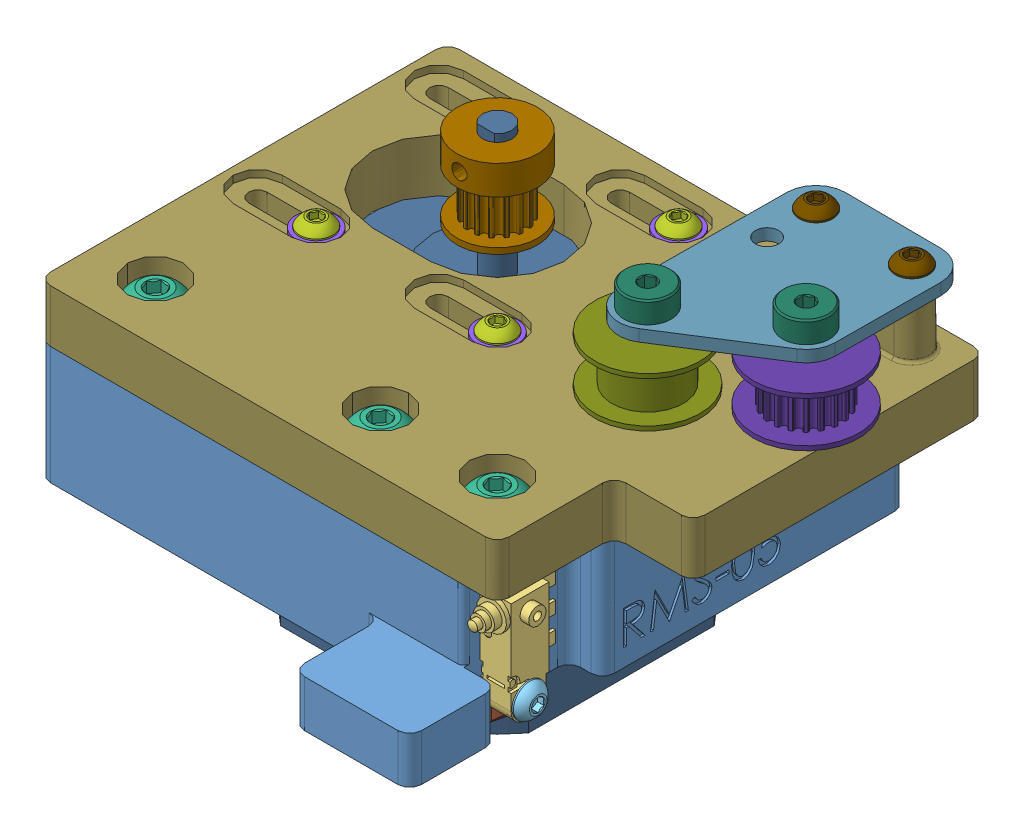
SolidWorks assembly right_motor_plate_assembly, configuration Default. Lengths in mm.
Overall size (94 73.14 85).
39 component instances, 18 part files, 47 mates.
Components (placement in the parent):
- tall_motor_corner_plate_spacer_assembly-1: tall_motor_corner_plate_spacer_assembly [Default] at (0 -0.4 -0.0001) x (1 0 0) z (0 0 1) size (82.91 20.2 85)
  - tall_motor_corner_plate_spacer_with_insert-1: tall_motor_corner_plate_spacer_with_insert [Default] at (354.071 392.0105 -198.139) x (0 0 -1) z (0 1 0) size (85 78.5 20.2)
    - motor_corner_bracket_spacer-1: motor_corner_bracket_spacer [Right Motor Corner Bracket Spacer] at (-213.4548 157 -10) x (0 -1 0) z (-1 0 0) size (78.5 20.2 85)
    - m4_heat_set_insert_long_94180A353-1: m4_heat_set_insert_long_94180A353 [94180A353] at (-165.9548 20 -4.5) x (0.989318 0 -0.145772) z (0.145772 0 0.989318) size (6.35 8.38 6.35)
  - D2HW_C201H-1: D2HW_C201H [Default] at (348.321 387.8105 9.5157) x (0 -1 0) z (-1 0 0) size (18.5 14.2 8.3)
  - m4_set_screw_25mm_92605A124-1: m4_set_screw_25mm_92605A124 [92605A124] at (345.571 387.5105 -32.1843) x (0 -0.291374 0.956609) z (1 0 0) size (4.62 4.11 25.58)
  - m3_8mm_buttonhead_screw_92095A181-1: m3_8mm_buttonhead_screw_92095A181 [92095A181] at (355.271 374.8105 9.5157) x (0 0 -1) z (1 0 0) size (5.7 5.7 9.95)
- m5_30mm_buttonhead_screw_92095A218-9: m5_30mm_buttonhead_screw_92095A218 [92095A218] at (344.0709 399.3605 5.3157) x (-0.927146 0 0.374699) z (0 1 0)
- m5_30mm_buttonhead_screw_92095A218-8: m5_30mm_buttonhead_screw_92095A218 [92095A218] at (324.0709 399.3605 5.3157) x (-0.927146 0 0.374699) z (0 1 0)
- m5_30mm_buttonhead_screw_92095A218-10: m5_30mm_buttonhead_screw_92095A218 [92095A218] at (285.5709 399.3605 5.3157) x (-0.917889 0 0.396837) z (0 1 0)
- m3_12mm_buttohead_screw_92095A183-1: m3_12mm_buttohead_screw_92095A183 [92095A183] at (291.071 401.6605 -47.6843) x (1 0 0) z (0 1 0)
- m3_stainless_steel_washer_90965A130-1: m3_stainless_steel_washer_90965A130 [90965A130] at (291.071 399.4105 -47.6843) x (0.988493 0 -0.151268) z (0 1 0)
- xy_drive_stepper-1: xy_drive_stepper [Default] at (334 7.6 0) x (1 0 0) z (0 0 1) size (42.42 72 42.42)
  - drive_pulley_16t_gt2_6mm_belt-1: drive_pulley_16t_gt2_6mm_belt [Default] at (-27.429 406.7309 -32.1843) x (-0.044306 0 -0.999018) z (-0.999018 0 0.044306) size (13.8 13.5 13.8)
  - 17HM19-2004S-1: 17HM19-2004S [Default] at (-27.429 384.0105 -32.1843) x (-1 0 0) z (0 1 0) size (42.42 42.42 72)
- m5_locking_t_nut_20x20_generic-1: m5_locking_t_nut_20x20_generic [Default] at (344.071 366.6105 -37.6843) x (-1 0 0) z (0 0 -1)
- m5_locking_t_nut_20x20_generic-2: m5_locking_t_nut_20x20_generic [Default] at (343.3974 366.6105 8.2391) x (-0.97447 0 -0.224516) z (0.224516 0 -0.97447)
- m5_locking_t_nut_20x20_generic-3: m5_locking_t_nut_20x20_generic [Default] at (288.5709 366.6105 5.3157) x (0 0 1) z (-1 0 0)
- m5_locking_t_nut_20x20_generic-5: m5_locking_t_nut_20x20_generic [Default] at (327.0709 366.6105 5.3157) x (0 0 1) z (-1 0 0)
- right_motor_plate_with_inserts-1: right_motor_plate_with_inserts [Default] at (0 -0.4 -0.0001) x (1 0 0) z (0 0 1) size (92 19.4 70)
  - motor_corner_bracket-1: motor_corner_bracket [Right Motor Corner Bracket] at (197.071 392.0105 15.3157) size (92 19.4 70)
  - m4_heat_set_insert_long_94180A353-1: m4_heat_set_insert_long_94180A353 [94180A353] at (360.571 401.0105 -31.0093) size (6.35 8.38 6.35)
  - m4_heat_set_insert_long_94180A353-2: m4_heat_set_insert_long_94180A353 [94180A353] at (344.071 401.0105 -20.3843) size (6.35 8.38 6.35)
- m5_shim_0.2mm_thick_98089A246-1: m5_shim_0.2mm_thick_98089A246 [98089A246] at (360.571 400.8105 -31.0093) x (0.674811 0 0.73799) z (0.73799 0 -0.674811)
- m5_shim_0.2mm_thick_98089A246-2: m5_shim_0.2mm_thick_98089A246 [98089A246] at (344.071 400.6105 -20.3843) x (-0.968571 0 0.248739) z (-0.248739 0 -0.968571)
- motor_plate_reinforcement-1: motor_plate_reinforcement [Default] at (365.699 413.0105 -53.9811) x (-0.999984 0 -0.005572) z (-0.005572 0 0.999984)
- m4_shoulder_screw_5mm_d_12mm_l_90278A371-1: m4_shoulder_screw_5mm_d_12mm_l_90278A371 [90278A371] at (360.571 416.6105 -31.0093) x (1 0 0) z (0 1 0)
- m4_shoulder_screw_5mm_d_12mm_l_90278A371-2: m4_shoulder_screw_5mm_d_12mm_l_90278A371 [90278A371] at (344.071 416.6105 -20.3843) x (1 0 0) z (0 1 0)
- 20t_toothless_idler_5mm_bore-1: 20t_toothless_idler_5mm_bore [Default] at (344.071 400.8105 -20.3843) x (0.998302 0 -0.058244) z (0.058244 0 0.998302)
- 20t_idler_5mm_bore-1: 20t_idler_5mm_bore [Default] at (360.571 400.8105 -31.0093)
- m3_6mm_buttonhead_screw_92095A179-1: m3_6mm_buttonhead_screw_92095A179 [92095A179] at (344.1715 414.6605 -49.1009) x (1 0 0) z (0 1 0)
- m3_6mm_buttonhead_screw_92095A179-2: m3_6mm_buttonhead_screw_92095A179 [92095A179] at (360.6712 414.6605 -49.009) x (1 0 0) z (0 1 0)
- m5_30mm_buttonhead_screw_92095A218-11: m5_30mm_buttonhead_screw_92095A218 [92095A218] at (344.071 399.3605 -40.6843) x (-0.971154 0 0.238453) z (0 1 0)
- m3_stainless_steel_washer_90965A130-2: m3_stainless_steel_washer_90965A130 [90965A130] at (322.071 399.4105 -47.6843) x (0.151268 0 0.988493) z (0 1 0)
- m3_stainless_steel_washer_90965A130-3: m3_stainless_steel_washer_90965A130 [90965A130] at (322.071 399.4105 -16.6843) x (-0.988493 0 0.151268) z (0 1 0)
- m3_stainless_steel_washer_90965A130-4: m3_stainless_steel_washer_90965A130 [90965A130] at (291.071 399.4105 -16.6843) x (-0.151268 0 -0.988493) z (0 1 0)
- m3_12mm_buttohead_screw_92095A183-2: m3_12mm_buttohead_screw_92095A183 [92095A183] at (322.071 401.6605 -47.6843) x (0 0 1) z (0 1 0)
- m3_12mm_buttohead_screw_92095A183-3: m3_12mm_buttohead_screw_92095A183 [92095A183] at (322.071 401.6605 -16.6843) x (-1 0 0) z (0 1 0)
- m3_12mm_buttohead_screw_92095A183-4: m3_12mm_buttohead_screw_92095A183 [92095A183] at (291.071 401.6605 -16.6843) x (0 0 -1) z (0 1 0)
Mates (geometry in assembly coordinates):
- Concentric754010197: concentric aligned: cylinder of m5_30mm_buttonhead_screw_92095A218-9 through (344.0709 399.3605 5.3157) axis (0 1 0) radius 4.75; cylinder of m5_locking_t_nut_20x20_generic-2 through (344.0709 371.1105 5.3157) axis (0 1 0) radius 2.1
- Coincident1594070768: coincident aligned: plane of m5_30mm_buttonhead_screw_92095A218-9 through (343.1342 366.6105 2.9979) normal (0 -1 0); plane of m5_locking_t_nut_20x20_generic-2 through (342.3083 366.6105 1.831) normal (0 -1 0)
- Concentric754010198: concentric aligned: cylinder of m5_30mm_buttonhead_screw_92095A218-8 through (324.0709 399.3605 5.3157) axis (0 1 0) radius 4.75; cylinder of m5_locking_t_nut_20x20_generic-5 through (324.0709 371.1105 5.3157) axis (0 1 0) radius 2.1
- Coincident1594070769: coincident aligned: plane of m5_30mm_buttonhead_screw_92095A218-8 through (323.1342 366.6105 2.9979) normal (0 -1 0); plane of m5_locking_t_nut_20x20_generic-5 through (321.0709 366.6105 7.8157) normal (0 -1 0)
- Concentric754010199: concentric aligned: circle of m5_30mm_buttonhead_screw_92095A218-5; cylinder of m5_locking_t_nut_20x20_generic-3 through (285.5709 371.1105 5.3157) axis (0 1 0) radius 2.1
- Coincident1594070770: coincident aligned: plane of m5_30mm_buttonhead_screw_92095A218-10 through (284.5789 366.6105 3.021) normal (0 -1 0); plane of m5_locking_t_nut_20x20_generic-3 through (282.5709 366.6105 7.8157) normal (0 -1 0)
- Concentric75400983: concentric aligned: cylinder of m4_shoulder_screw_5mm_d_12mm_l_90278A371-1 through (360.571 395.6105 -31.0093) axis (0 -1 0) radius 2.5; circle of motor_plate_reinforcement-1
- Concentric7540099451: concentric aligned: cylinder of motor_plate_reinforcement-1 through (344.1715 411.0105 -49.1009) axis (0 1 0) radius 1.6; cylinder of m3_6mm_buttonhead_screw_92095A179-1 through (344.1715 414.6605 -49.1009) axis (0 1 0) radius 2.85
- Coincident15940704882: coincident anti-aligned: plane of motor_plate_reinforcement-1 through (365.699 413.0105 -53.9811) normal (0 1 0); plane of m3_6mm_buttonhead_screw_92095A179-1 through (344.1715 413.0105 -46.2509) normal (0 -1 0)
- Concentric7540099461: concentric aligned: cylinder of motor_plate_reinforcement-1 through (360.6712 411.0105 -49.009) axis (0 1 0) radius 1.6; cylinder of m3_6mm_buttonhead_screw_92095A179-2 through (360.6712 414.6605 -49.009) axis (0 1 0) radius 2.85
- Coincident15940704892: coincident anti-aligned: plane of motor_plate_reinforcement-1 through (365.699 413.0105 -53.9811) normal (0 1 0); plane of m3_6mm_buttonhead_screw_92095A179-2 through (360.6712 413.0105 -46.159) normal (0 -1 0)
- Concentric754009959: concentric anti-aligned: cylinder of m4_shoulder_screw_5mm_d_12mm_l_90278A371-2 through (344.071 395.6105 -20.3843) axis (0 -1 0) radius 2.5; circle of m5_shim_0.2mm_thick_98089A246-2
- Concentric7540099191: concentric anti-aligned: cylinder of m3_stainless_steel_washer_90965A130-1 through (291.071 400.0105 -47.6843) axis (0 -1 0) radius 1.6; cylinder of m3_12mm_buttohead_screw_92095A183-1 through (291.071 401.6605 -47.6843) axis (0 1 0) radius 2.85
- Coincident15940704891: coincident anti-aligned: plane of m3_stainless_steel_washer_90965A130-1 through (291.071 400.0105 -47.6843) normal (0 1 0); plane of m3_12mm_buttohead_screw_92095A183-1 through (291.071 400.0105 -44.8343) normal (0 -1 0)
- Concentric754010289: concentric aligned: cylinder of m5_30mm_buttonhead_screw_92095A218-11 through (344.071 399.3605 -40.6843) axis (0 1 0) radius 4.75; cylinder of m5_locking_t_nut_20x20_generic-1 through (344.071 371.1105 -40.6843) axis (0 1 0) radius 2.1
- Coincident1594070880: coincident aligned: plane of m5_30mm_buttonhead_screw_92095A218-11 through (343.4748 366.6105 -43.1122) normal (0 -1 0); plane of m5_locking_t_nut_20x20_generic-1 through (341.571 366.6105 -43.6843) normal (0 -1 0)
- Concentric754010288: concentric aligned: cylinder of m4_shoulder_screw_5mm_d_12mm_l_90278A371-2 through (344.071 395.6105 -20.3843) axis (0 -1 0) radius 2.5; cylinder of 20t_toothless_idler_5mm_bore-1 through (344.071 400.8105 -20.3843) axis (0 -1 0) radius 6.1
- Coincident1594070882: coincident anti-aligned: plane of m5_shim_0.2mm_thick_98089A246-2 through (344.071 400.8105 -20.3843) normal (0 1 0); plane of 20t_toothless_idler_5mm_bore-1 through (353.0557 400.8105 -20.9085) normal (0 -1 0)
- Concentric754010287: concentric aligned: cylinder of m4_shoulder_screw_5mm_d_12mm_l_90278A371-1 through (360.571 395.6105 -31.0093) axis (0 -1 0) radius 2.5; circle of 20t_idler_5mm_bore-1
- Coincident1594070881: coincident anti-aligned: plane of m5_shim_0.2mm_thick_98089A246-1 through (360.571 400.8105 -31.0093) normal (0 1 0); plane of 20t_idler_5mm_bore-1 through (369.571 400.8105 -31.0093) normal (0 -1 0)
- Concentric754010298: concentric anti-aligned: cylinder of right_motor_plate_with_inserts-1/motor_corner_bracket-1 through (344.0709 400.6105 5.3157) axis (0 -1 0) radius 2.6; cylinder of m5_30mm_buttonhead_screw_92095A218-9 through (344.0709 399.3605 5.3157) axis (0 1 0) radius 4.75
- Coincident1594070892: coincident aligned: plane of right_motor_plate_with_inserts-1/motor_corner_bracket-1 through (344.0709 396.6105 5.3157) normal (0 1 0); circle of m5_30mm_buttonhead_screw_92095A218-6
- Concentric754010299: concentric anti-aligned: cylinder of right_motor_plate_with_inserts-1/motor_corner_bracket-1 through (324.0709 400.6105 5.3157) axis (0 -1 0) radius 2.6; cylinder of m5_30mm_buttonhead_screw_92095A218-8 through (324.0709 399.3605 5.3157) axis (0 1 0) radius 4.75
- Coincident1594070893: coincident aligned: plane of right_motor_plate_with_inserts-1/motor_corner_bracket-1 through (324.0709 396.6105 5.3157) normal (0 1 0); circle of m5_30mm_buttonhead_screw_92095A218-7
- Concentric754010300: concentric anti-aligned: cylinder of right_motor_plate_with_inserts-1/motor_corner_bracket-1 through (285.5709 400.6105 5.3157) axis (0 -1 0) radius 2.6; circle of m5_30mm_buttonhead_screw_92095A218-5
- Coincident1594070894: coincident aligned: plane of right_motor_plate_with_inserts-1/motor_corner_bracket-1 through (285.5709 396.6105 5.3157) normal (0 1 0); circle of m5_30mm_buttonhead_screw_92095A218-5
- Coincident1594070895: coincident anti-aligned: plane of right_motor_plate_with_inserts-1/motor_corner_bracket-1 through (360.571 411.0105 -49.0093) normal (0 1 0); plane of motor_plate_reinforcement-1 through (365.699 411.0105 -53.9811) normal (0 -1 0)
- Concentric754010301: concentric aligned: cylinder of right_motor_plate_with_inserts-1/motor_corner_bracket-1 through (360.571 400.6105 -31.0093) axis (0 -1 0) radius 2.7; cone of m4_shoulder_screw_5mm_d_12mm_l_90278A371-1 through (360.571 400.6105 -31.0093) axis (0 -1 0)
- Coincident1594070896: coincident anti-aligned: plane of right_motor_plate_with_inserts-1/motor_corner_bracket-1 through (354.0709 400.6105 15.3157) normal (0 1 0); plane of m4_shoulder_screw_5mm_d_12mm_l_90278A371-1 through (360.571 400.6105 -28.5093) normal (0 -1 0)
- Concentric754010302: concentric aligned: cylinder of right_motor_plate_with_inserts-1/motor_corner_bracket-1 through (344.071 400.6105 -20.3843) axis (0 -1 0) radius 2.7; cone of m4_shoulder_screw_5mm_d_12mm_l_90278A371-2 through (344.071 400.6105 -20.3843) axis (0 -1 0)
- Coincident1594070897: coincident anti-aligned: plane of right_motor_plate_with_inserts-1/motor_corner_bracket-1 through (354.0709 400.6105 15.3157) normal (0 1 0); plane of m4_shoulder_screw_5mm_d_12mm_l_90278A371-2 through (344.071 400.6105 -17.8843) normal (0 -1 0)
- Concentric754010303: concentric aligned: cylinder of right_motor_plate_with_inserts-1/motor_corner_bracket-1 through (291.071 400.6105 -47.6843) axis (0 -1 0) radius 1.6; cylinder of m3_stainless_steel_washer_90965A130-1 through (291.071 400.0105 -47.6843) axis (0 -1 0) radius 3.5
- Coincident1594070898: coincident anti-aligned: plane of right_motor_plate_with_inserts-1/motor_corner_bracket-1 through (291.071 399.4105 -47.6843) normal (0 1 0); plane of m3_stainless_steel_washer_90965A130-1 through (291.071 399.4105 -47.6843) normal (0 -1 0)
- Coincident1594070899: coincident anti-aligned: plane of right_motor_plate_with_inserts-1/motor_corner_bracket-1 through (354.0709 391.6105 15.3157) normal (0 -1 0); plane of xy_drive_stepper-1/17HM19-2004S-1 through (306.571 391.6105 -32.1843) normal (0 1 0)
- Concentric754010304: concentric anti-aligned: circle of right_motor_plate_with_inserts-1/motor_corner_bracket-1; circle of xy_drive_stepper-1/17HM19-2004S-1
- Concentric754010305: concentric aligned: cylinder of right_motor_plate_with_inserts-1/motor_corner_bracket-1 through (306.571 400.6105 -32.1843) axis (0 -1 0) radius 11.4; circle of xy_drive_stepper-1/17HM19-2004S-1
- Concentric754010306: concentric anti-aligned: cylinder of right_motor_plate_with_inserts-1/motor_corner_bracket-1 through (360.571 400.6105 -31.0093) axis (0 -1 0) radius 2.7; cylinder of m5_shim_0.2mm_thick_98089A246-1 through (360.571 400.6105 -31.0093) axis (0 1 0) radius 5
- Coincident1594070900: coincident anti-aligned: plane of right_motor_plate_with_inserts-1/motor_corner_bracket-1 through (354.0709 400.6105 15.3157) normal (0 1 0); plane of m5_shim_0.2mm_thick_98089A246-1 through (360.571 400.6105 -31.0093) normal (0 -1 0)
- Coincident1594070901: coincident anti-aligned: plane of right_motor_plate_with_inserts-1/motor_corner_bracket-1 through (354.0709 400.6105 15.3157) normal (0 1 0); plane of m5_shim_0.2mm_thick_98089A246-2 through (344.071 400.6105 -20.3843) normal (0 -1 0)
- Concentric754010307: concentric anti-aligned: cylinder of right_motor_plate_with_inserts-1/motor_corner_bracket-1 through (344.071 400.6105 -40.6843) axis (0 -1 0) radius 2.6; cylinder of m5_30mm_buttonhead_screw_92095A218-11 through (344.071 399.3605 -40.6843) axis (0 1 0) radius 4.75
- Coincident1594070902: coincident aligned: plane of right_motor_plate_with_inserts-1/motor_corner_bracket-1 through (344.071 396.6105 -40.6843) normal (0 1 0); circle of m5_30mm_buttonhead_screw_92095A218-4
- Parallel56: parallel aligned: plane of tall_motor_corner_plate_spacer_assembly-1/tall_motor_corner_plate_spacer_with_insert-1/motor_corner_bracket_spacer-1 through (334.071 391.6105 -54.6843) normal (0 0 -1); plane of m5_locking_t_nut_20x20_generic-1 through (344.071 366.6105 -43.6843) normal (0 0 -1)
- Parallel57: parallel aligned: plane of tall_motor_corner_plate_spacer_assembly-1/tall_motor_corner_plate_spacer_with_insert-1/motor_corner_bracket_spacer-1 through (354.071 391.6105 -54.6843) normal (1 0 0); plane of m5_locking_t_nut_20x20_generic-3 through (288.5709 366.6105 5.3157) normal (1 0 0)
- Parallel58: parallel aligned: plane of tall_motor_corner_plate_spacer_assembly-1/tall_motor_corner_plate_spacer_with_insert-1/motor_corner_bracket_spacer-1 through (354.071 391.6105 -54.6843) normal (1 0 0); plane of m5_locking_t_nut_20x20_generic-5 through (327.0709 366.6105 5.3157) normal (1 0 0)
- Coincident1594070906: coincident aligned: plane of right_motor_plate_with_inserts-1/motor_corner_bracket-1 through (354.0709 400.6105 15.3157) normal (0 0 1); plane of tall_motor_corner_plate_spacer_assembly-1/tall_motor_corner_plate_spacer_with_insert-1/motor_corner_bracket_spacer-1 through (354.0709 391.6105 15.3157) normal (0 0 1)
- Coincident1594070907: coincident aligned: plane of right_motor_plate_with_inserts-1/motor_corner_bracket-1 through (354.071 400.6105 -4.6843) normal (1 0 0); plane of tall_motor_corner_plate_spacer_assembly-1/tall_motor_corner_plate_spacer_with_insert-1/motor_corner_bracket_spacer-1 through (354.071 391.6105 -54.6843) normal (1 0 0)
- Coincident1594070908: coincident anti-aligned: plane of right_motor_plate_with_inserts-1/motor_corner_bracket-1 through (354.0709 391.6105 15.3157) normal (0 -1 0); plane of tall_motor_corner_plate_spacer_assembly-1/tall_motor_corner_plate_spacer_with_insert-1/motor_corner_bracket_spacer-1 through (354.0709 391.6105 15.3157) normal (0 1 0)
